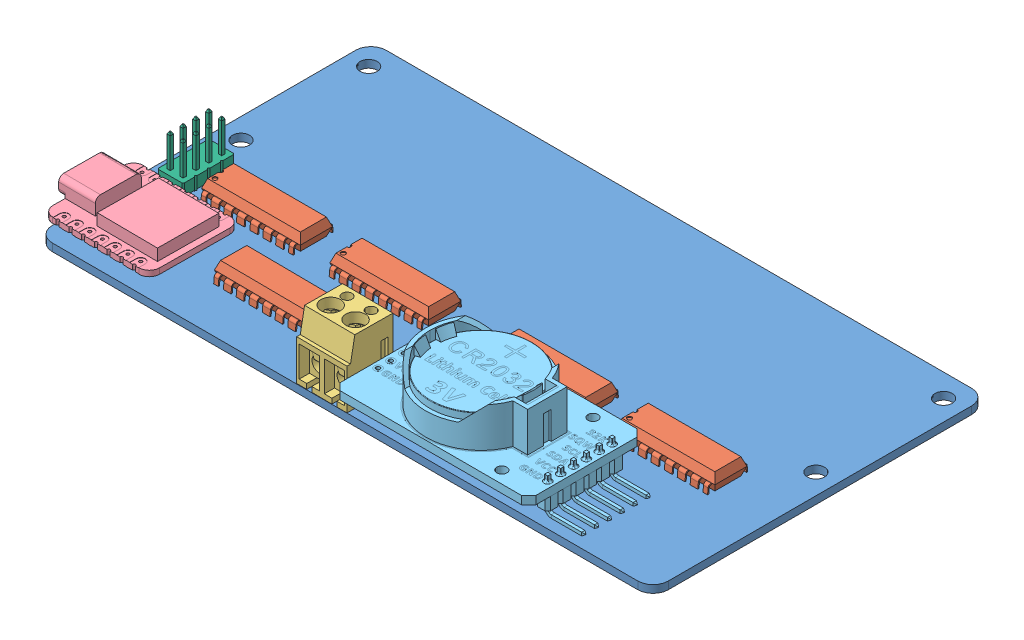
SolidWorks assembly board2, configuration Défaut. Lengths in mm.
Overall size (122.67 19.21 69.85).
11 component instances, 6 part files, 16 mates.
Components (placement in the parent):
- pcb-1: pcb [Défaut] at origin size (121.6 1.5 65.9)
- DIP18N.step-1: DIP18N.step [Défaut] at (-50.7835 3.7087 35.4382) x (0 0 1) z (-1 0 0) size (8.53 6.85 19.5)
- DIP18N.step-2: DIP18N.step [Défaut] at (31.1067 3.7087 35.4997) x (0 0 1) z (-1 0 0) size (8.53 6.85 19.5)
- DIP18N.step-3: DIP18N.step [Défaut] at (5.6608 3.7087 35.5611) x (0 0 1) z (-1 0 0) size (8.53 6.85 19.5)
- DIP18N.step-4: DIP18N.step [Défaut] at (-25.3559 3.7087 35.5399) x (0 0 1) z (-1 0 0) size (8.53 6.85 19.5)
- DIP18N.step-5: DIP18N.step [Défaut] at (-15.751 3.7087 -7.8923) x (0.008727 0 -0.999962) z (0.999962 0 0.008727) size (8.53 6.85 19.5)
- DIP18N.step-6: DIP18N.step [Défaut] at (34.3108 3.7087 -7.8662) x (0.008727 0 -0.999962) z (0.999962 0 0.008727) size (8.53 6.85 19.5)
- Screw Terminal Block 5mm-2: Screw Terminal Block 5mm [Valor predeterminado] at (0.4217 1.5 23.933) x (-0.999962 0 -0.008727) z (0.008727 0 -0.999962) size (10.6 16.9 9)
- Seeeduino Xiao.step-1: Seeeduino Xiao.step [Défaut] at (-88.5187 11.44 25.9289) x (-0.008727 0 0.999962) z (-0.999962 0 -0.008727) size (17.8 4.27 22.5)
- DS3231 RTC.step-1: DS3231 RTC.step [Défaut] at (20.896 7 25.5045) x (-1 0 0) z (0 -1 0) size (44.75 22.8 13.53)
- zl202-8_p2-54_l10-2_w5-08_h8-89.stp-1: zl202-8_p2-54_l10-2_w5-08_h8-89.stp [Défaut] at (-55.033 1.5 3.5455) x (0 0 1) z (-1 0 0) size (10.16 11.94 5.08)
Mates (geometry in assembly coordinates):
- Coïncidente15: coincident anti-aligned: plane of pcb-1 through (0 1.5 0) normal (0 1 0); plane of DIP18N.step-1 through (-31.2835 1.5 4.7548) normal (0 -1 0)
- Coïncidente16: coincident anti-aligned: plane of pcb-1 through (0 1.5 0) normal (0 1 0); plane of DIP18N.step-4 through (-5.8559 1.5 4.8565) normal (0 -1 0)
- Coïncidente17: coincident anti-aligned: plane of pcb-1 through (0 1.5 0) normal (0 1 0); plane of DIP18N.step-3 through (25.1608 1.5 4.8776) normal (0 -1 0)
- Coïncidente18: coincident anti-aligned: plane of pcb-1 through (0 1.5 0) normal (0 1 0); plane of DIP18N.step-2 through (50.6067 1.5 4.8163) normal (0 -1 0)
- Coïncidente21: coincident anti-aligned: plane of pcb-1 through (0 1.5 0) normal (0 1 0); plane of DIP18N.step-5 through (-35.5181 1.5 22.6198) normal (0 -1 0)
- Coïncidente22: coincident anti-aligned: plane of pcb-1 through (0 1.5 0) normal (0 1 0); plane of DIP18N.step-6 through (14.5438 1.5 22.6458) normal (0 -1 0)
- Coïncidente23: coincident anti-aligned: plane of pcb-1 through (0 1.5 0) normal (0 1 0); plane of Screw Terminal Block 5mm-2 through (-9.6565 1.5 32.8454) normal (0 -1 0)
- Distance1: distance = 2.5 mm anti-aligned: plane of Seeeduino Xiao.step-1 through (-49.894 4 23.2659) normal (0 -1 0); plane of pcb-1 through (0 1.5 0) normal (0 1 0)
- Coïncidente26: coincident aligned: plane of pcb-1 through (0 0 0) normal (1 0 0)
- Coïncidente27: coincident aligned: plane of pcb-1 through (0 0 0) normal (0 0 1)
- Coïncidente28: coincident aligned: plane of pcb-1 through (0 0 0) normal (0 1 0)
- Parallèle8: parallel aligned: plane of pcb-1 through (0 0 0) normal (0 -1 0); plane of DS3231 RTC.step-1 through (20.896 7 25.5045) normal (0 -1 0)
- Distance2: distance = 5.5 mm anti-aligned: plane of pcb-1 through (0 1.5 0) normal (0 1 0); plane of DS3231 RTC.step-1 through (20.896 7 25.5045) normal (0 -1 0)
- Parallèle9: parallel aligned: plane of pcb-1 through (-60.8 1.5 32.95) normal (0 0 1); plane of DS3231 RTC.step-1 through (40.196 8.6 36.9045) normal (0 0 1)
- Coïncidente30: coincident anti-aligned: plane of pcb-1 through (0 1.5 0) normal (0 1 0); plane of zl202-8_p2-54_l10-2_w5-08_h8-89.stp-1 through (-55.033 1.5 3.5455) normal (0 -1 0)
- Parallèle11: parallel aligned: plane of pcb-1 through (-60.8 1.5 -32.95) normal (-1 0 0); plane of zl202-8_p2-54_l10-2_w5-08_h8-89.stp-1 through (-57.573 1.5 5.0695) normal (-1 0 0)
